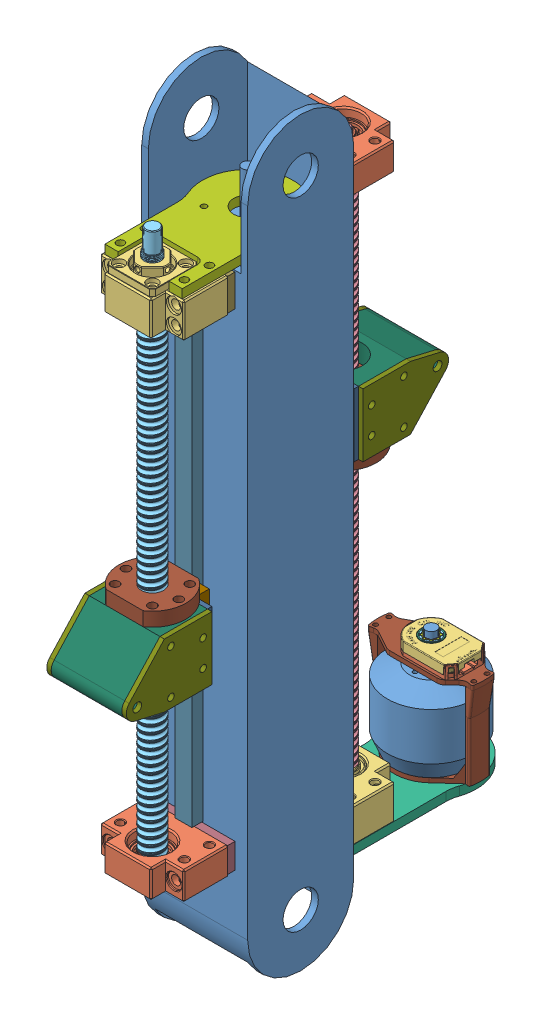
SolidWorks assembly Shoulder, configuration Default. Lengths in mm.
Overall size (98.94 533.4 280.38).
61 component instances, 29 part files, 54 mates.
Components (placement in the parent):
- Box^Shoulder-1: Box^Shoulder [Default] at origin size (76.2 533.4 76.2) (virtual)
- BF12-1: BF12 [Default] at (0 590.6294 -38.2263) x (1 0 0) z (0 1 0) size (60 43 20)
- BK12-1: BK12 [Default] at (0 188.6294 -38.2263) x (-1 0 0) z (0 -1 0) size (60 46.94 35.34)
- SFU1605-450-1: SFU1605-450 [1605-400] at (0 147.6294 -63.2263) x (1 0 0) z (0 -1 0) size (16.38 16.22 450)
- BK12-2: BK12 [Default] at (0 563.5294 48.7687) x (-1 0 0) z (0 1 0) size (60 46.94 35.34)
- BF12-2: BF12 [Default] at (0 211.5294 48.7687) x (-1 0 0) z (0 1 0) size (60 43 20)
- SFU1605-400-3: SFU1605-400 [1605-400] at (0 604.5294 73.7687) x (-1 0 0) z (0 1 0) size (16.52 16.22 400)
- J3Plate^Shoulder-1: J3Plate^Shoulder [Default] at origin size (65 6.35 120.35) (virtual)
- J2Plate^Shoulder-1: J2Plate^Shoulder [Default] at origin size (65 6.35 107.35) (virtual)
- J3MGN12R-1: J3MGN12R [Default] at origin size (12 379.5 8)
- J3MGN12C-1: J3MGN12C [Default] at (0 433.1293 -40.8288) x (1 0 0) z (0 1 0) size (27 10 45.5)
- CarriagePlate^Shoulder-1: CarriagePlate^Shoulder [Default] at (0 67.1524 5.2712) size (50.8 45.5 3.17) (virtual)
- nut-1: nut [Default] at (0 410.3793 -63.2263) x (-1 0 0) z (0 -1 0) size (48 40 42)
- BKSpacer^Shoulder-1: BKSpacer^Shoulder [Default] at origin size (58 23 5.4) (virtual)
- BKSpacer^Shoulder-2: BKSpacer^Shoulder [Default] at (0 374.9 81.5975) size (58 23 5.4) (virtual)
- BFSpacer^Shoulder-1: BFSpacer^Shoulder [Default] at origin size (58 18 5.4) (virtual)
- BFSpacer^Shoulder-2: BFSpacer^Shoulder [Default] at (0 -379.1 81.5975) size (58 18 5.4) (virtual)
- J2MGN12R^Shoulder-1: J2MGN12R^Shoulder [Default] at origin size (12 329.5 8) (virtual)
- Adapter^Shoulder-2: Adapter^Shoulder [Default] at (0 76.5186 5.2712) size (57.15 45.79 61.61) (virtual)
  - Body^Adapter_Shoulder-1: Body^Adapter_Shoulder [Default] at (38.1 26.927 0) x (0 0 -1) z (1 0 0) size (61.61 45.5 50.8) (virtual)
  - SidePlate^Adapter_Shoulder-1: SidePlate^Adapter_Shoulder [Default] at origin size (3.18 45.5 61.61) (virtual)
  - SidePlate^Adapter_Shoulder-2: SidePlate^Adapter_Shoulder [Default] at (53.975 0 0) size (3.18 45.5 61.61) (virtual)
  - 94459A340_BRASS HEAT-SET INSERT FOR PLASTIC-1: 94459A340_BRASS HEAT-SET INSERT FOR PLASTIC [94459A340] at (-18.415 340.7357 -83.735) x (0 -1 0) z (0 0 -1) size (7.22 6.55 7.22)
  - 94459A220_BRASS HEAT-SET INSERT FOR PLASTIC-1: 94459A220_BRASS HEAT-SET INSERT FOR PLASTIC [94459A220] at (13.435 346.5607 -81.9325) x (-0.837169 0 -0.546944) z (-0.546944 0 0.837169) size (8.76 13.2 8.76)
- J3MGN12C-2: J3MGN12C [Default] at (0 348.7149 51.3712) x (-1 0 0) z (0 1 0) size (27 10 45.5)
- nut-2: nut [Default] at (0 371.4649 73.7687) x (1 0 0) z (0 1 0) size (48 40 42)
- Adapter^Shoulder-3: Adapter^Shoulder [Default] at (0 705.3256 5.2712) x (1 0 0) z (0 0 -1) size (57.15 45.79 61.61) (virtual)
  - Body^Adapter_Shoulder-1: Body^Adapter_Shoulder [Default] at (38.1 26.927 0) x (0 0 -1) z (1 0 0) size (61.61 45.5 50.8) (virtual)
  - SidePlate^Adapter_Shoulder-1: SidePlate^Adapter_Shoulder [Default] at origin size (3.18 45.5 61.61) (virtual)
  - SidePlate^Adapter_Shoulder-2: SidePlate^Adapter_Shoulder [Default] at (53.975 0 0) size (3.18 45.5 61.61) (virtual)
  - 94459A340_BRASS HEAT-SET INSERT FOR PLASTIC-1: 94459A340_BRASS HEAT-SET INSERT FOR PLASTIC [94459A340] at (-18.415 340.7357 -83.735) x (0 -1 0) z (0 0 -1) size (7.22 6.55 7.22)
  - 94459A220_BRASS HEAT-SET INSERT FOR PLASTIC-1: 94459A220_BRASS HEAT-SET INSERT FOR PLASTIC [94459A220] at (13.435 346.5607 -81.9325) x (-0.837169 0 -0.546944) z (-0.546944 0 0.837169) size (8.76 13.2 8.76)
- CarriagePlate^Shoulder-2: CarriagePlate^Shoulder [Default] at (0 -17.262 5.2712) x (-1 0 0) z (0 0 -1) size (50.8 45.5 3.17) (virtual)
- MotorEncoded-1: MotorEncoded [Default] at (0 179.3044 -126.7263) x (0 0 -1) z (1 0 0) size (63 110 76.93)
  - BetterKEDA-1: BetterKEDA [Default] at origin size (63 110 63)
  - CUI_DEVICES_AMT102-0048-N2000-S-1: CUI_DEVICES_AMT102-0048-N2000-S [Default] at (0 65.12 0) x (1 0 0) z (0 1 0) size (36.33 46.21 9.2)
    - CUI_DEVICES_AMT102-0048-N2000-S.step-1: CUI_DEVICES_AMT102-0048-N2000-S.step [Default] at origin size (36.33 46.21 9.2)
      - AMT-102-Base-REV-K.step-1: AMT-102-Base-REV-K.step [Default] x (-1 0 0) z (0 0 -1) size (28.78 43.39 9.06)
      - AMT-102-Top-Cover-REV-H.step-1: AMT-102-Top-Cover-REV-H.step [Default] at (0 0 5.23) x (-1 0 0) z (0 0 -1) size (28.6 43.26 6.55)
      - AMT-Sleeve-REV-D_ 2 mm.step-1: AMT-Sleeve-REV-D_ 2 mm.step [Default] at (0 0 -2.42) x (0.999996 0.002864 0) z (0 0 1) size (10.79 10.79 7.8)
      - AMT-Hub-Top-REV-D1.step-1: AMT-Hub-Top-REV-D1.step [Default] at (0 0 2.13) x (0.999996 0.002864 0) z (0 0 1) size (14 14 5.67)
      - AMT-Hub-Bottom-REV-B.step-1: AMT-Hub-Bottom-REV-B.step [Default] at (0 0 2.43) x (0.999998 -0.001942 0) z (0 0 1) size (17.3 17.3 3.2)
      - AMT10X-Shaft-Adaptor-REV-E.step-1: AMT10X-Shaft-Adaptor-REV-E.step [Default] at (0 0 0.03) x (0.999996 0.002864 0) z (0 0 1) size (11.8 11.8 7.8)
      - Receiver-board.step-1: Receiver-board.step [Default] at (72.2834 -20.351 3.03) x (-1 0 0) z (0 0 -1) size (26.5 26.62 0.41)
      - Rotor-board-REV F.step-1: Rotor-board-REV F.step [Default] at (0 0 2.13) x (0.807874 -0.589355 0) z (0 0 1) size (26 26 0.3)
      - Transmitter-board AMT10_AMT-102.step-1: Transmitter-board AMT10_AMT-102.step [Default] at (19.1596 -17.1102 1.22) x (-1 0 0) z (0 0 -1) size (26.63 38.43 4.41)
  - Body^MotorEncoded-1: Body^MotorEncoded [Default] at origin size (53 64.53 76.93) (virtual)
- MotorEncoded-2: MotorEncoded [Default] at (0 572.8544 5.2712) x (-0.707107 0 -0.707107) z (-0.707107 0 0.707107) size (63 110 76.93)
  - BetterKEDA-1: BetterKEDA [Default] at origin size (63 110 63)
  - CUI_DEVICES_AMT102-0048-N2000-S-1: CUI_DEVICES_AMT102-0048-N2000-S [Default] at (0 65.12 0) x (1 0 0) z (0 1 0) size (36.33 46.21 9.2)
    - CUI_DEVICES_AMT102-0048-N2000-S.step-1: CUI_DEVICES_AMT102-0048-N2000-S.step [Default] at origin size (36.33 46.21 9.2)
      - AMT-102-Base-REV-K.step-1: AMT-102-Base-REV-K.step [Default] x (-1 0 0) z (0 0 -1) size (28.78 43.39 9.06)
      - AMT-102-Top-Cover-REV-H.step-1: AMT-102-Top-Cover-REV-H.step [Default] at (0 0 5.23) x (-1 0 0) z (0 0 -1) size (28.6 43.26 6.55)
      - AMT-Sleeve-REV-D_ 2 mm.step-1: AMT-Sleeve-REV-D_ 2 mm.step [Default] at (0 0 -2.42) x (0.999996 0.002864 0) z (0 0 1) size (10.79 10.79 7.8)
      - AMT-Hub-Top-REV-D1.step-1: AMT-Hub-Top-REV-D1.step [Default] at (0 0 2.13) x (0.999996 0.002864 0) z (0 0 1) size (14 14 5.67)
      - AMT-Hub-Bottom-REV-B.step-1: AMT-Hub-Bottom-REV-B.step [Default] at (0 0 2.43) x (0.999998 -0.001942 0) z (0 0 1) size (17.3 17.3 3.2)
      - AMT10X-Shaft-Adaptor-REV-E.step-1: AMT10X-Shaft-Adaptor-REV-E.step [Default] at (0 0 0.03) x (0.999996 0.002864 0) z (0 0 1) size (11.8 11.8 7.8)
      - Receiver-board.step-1: Receiver-board.step [Default] at (72.2834 -20.351 3.03) x (-1 0 0) z (0 0 -1) size (26.5 26.62 0.41)
      - Rotor-board-REV F.step-1: Rotor-board-REV F.step [Default] at (0 0 2.13) x (0.807874 -0.589355 0) z (0 0 1) size (26 26 0.3)
      - Transmitter-board AMT10_AMT-102.step-1: Transmitter-board AMT10_AMT-102.step [Default] at (19.1596 -17.1102 1.22) x (-1 0 0) z (0 0 -1) size (26.63 38.43 4.41)
  - Body^MotorEncoded-1: Body^MotorEncoded [Default] at origin size (53 64.53 76.93) (virtual)
Mates (geometry in assembly coordinates):
- Parallel1: parallel anti-aligned: plane of Box^Shoulder-1 through (-33.3375 163.4294 -32.8288) normal (0 0 -1); plane of BF12-1 through (29 581.6294 -38.2263) normal (0 0 1)
- Width1: width anti-aligned: plane of BF12-1 through (30 581.6294 -69.7263) normal (1 0 0); plane of BF12-1 through (-30 581.6294 -39.2263) normal (-1 0 0); plane of Box^Shoulder-1 through (38.1 620.6294 5.2712) normal (1 0 0); plane of Box^Shoulder-1 through (-38.1 163.4294 5.2712) normal (-1 0 0)
- Distance6: distance anti-aligned: plane of Box^Shoulder-1 through (-33.3375 163.4294 -32.8288) normal (0 0 -1); plane of BK12-1 through (-29 200.1294 -38.2263) normal (0 0 1)
- Width2: width aligned: plane of BK12-1 through (30 200.1294 -39.2263) normal (1 0 0); plane of BK12-1 through (-30 200.1294 -69.7263) normal (-1 0 0); plane of Box^Shoulder-1 through (-38.1 163.4294 5.2712) normal (-1 0 0); plane of Box^Shoulder-1 through (38.1 620.6294 5.2712) normal (1 0 0)
- Parallel3: parallel aligned: plane of BK12-1 through (29 201.1294 -39.2263) normal (0 1 0)
- Coincident11: coincident: line of SFU1605-450-1 through (0 162.3794 -63.2263) axis (0 -1 0)
- Concentric6: concentric anti-aligned: cylinder of BK12-1 through (0 196.6294 -63.2263) axis (0 1 0) radius 6; cylinder of SFU1605-450-1 through (0 162.6294 -63.2263) axis (0 -1 0) radius 5
- Coincident12: coincident anti-aligned: plane of BK12-1 through (7.2358 201.6294 -55.9905) normal (0 1 0); plane of SFU1605-450-1 through (0 201.6294 -63.2263) normal (0 -1 0)
- Coincident13: coincident anti-aligned: plane of BF12-1 through (-6.5021 586.6294 -56.7242) normal (0 -1 0); plane of SFU1605-450-1 through (0 586.6294 -63.2263) normal (0 1 0)
- Distance3: distance = 12.7 mm: plane of BK12-1 through (29 176.1294 -39.2263) normal (0 -1 0); line of Box^Shoulder-1 through (38.1 163.4294 -32.8288) axis (-1 0 0)
- Coincident27: coincident: line of SFU1605-400-3 through (0 589.7794 73.7687) axis (0 1 0)
- Concentric18: concentric anti-aligned: cylinder of BK12-2 through (0 563.5294 73.7687) axis (0 -1 0) radius 6; cylinder of SFU1605-400-3 through (0 589.5294 73.7687) axis (0 1 0) radius 5
- Distance8: distance anti-aligned: plane of Box^Shoulder-1 through (-33.3375 163.4294 43.3712) normal (0 0 1); plane of BK12-2 through (-29 552.0294 48.7687) normal (0 0 -1)
- Coincident29: coincident anti-aligned: plane of BK12-2 through (7.2358 550.5294 66.5329) normal (0 -1 0); plane of SFU1605-400-3 through (0 550.5294 73.7687) normal (0 1 0)
- Coincident30: coincident anti-aligned: plane of BF12-2 through (-6.5021 215.5294 67.2666) normal (0 1 0); plane of SFU1605-400-3 through (0 215.5294 73.7687) normal (0 -1 0)
- Concentric19: concentric anti-aligned: cylinder of BF12-2 through (0 208.3294 73.7687) axis (0 1 0) radius 5; cylinder of SFU1605-400-3 through (0 215.5294 73.7687) axis (0 -1 0) radius 5
- Distance5: distance = 38.1 mm: line of Box^Shoulder-1 through (38.1 163.4294 43.3712) axis (-1 0 0); plane of BF12-2 through (29 201.5294 49.7687) normal (0 -1 0)
- Coincident35: coincident anti-aligned: plane of J3MGN12R-1 through (0 0 -40.8288) normal (0 0 -1); plane of J3MGN12C-1 through (-6 455.8793 -40.8288) normal (0 0 1)
- Width3: width anti-aligned: plane of J3MGN12C-1 through (13.5 455.8793 -35.8288) normal (1 0 0); plane of J3MGN12R-1 through (-13.5 455.8793 -35.8288) normal (-1 0 0); plane of J3MGN12C-1 through (-6 580.6294 -40.8288) normal (-1 0 0); plane of J3MGN12R-1 through (6 580.6294 -40.8288) normal (1 0 0)
- Coincident36: coincident anti-aligned: plane of J3MGN12C-1 through (13.5 455.8793 -45.8288) normal (0 0 -1); plane of CarriagePlate^Shoulder-1 through (0 67.1524 -45.8288) normal (0 0 1)
- Concentric22: concentric anti-aligned: cylinder of J3MGN12C-1 through (10 443.1293 -41.8288) axis (0 0 -1) radius 1.5; cylinder of CarriagePlate^Shoulder-1 through (10 443.1293 -49.0038) axis (0 0 1) radius 1.5
- Concentric23: concentric anti-aligned: cylinder of J3MGN12C-1 through (-10 423.1293 -41.8288) axis (0 0 -1) radius 1.5; cylinder of CarriagePlate^Shoulder-1 through (-10 423.1293 -49.0038) axis (0 0 1) radius 1.5
- Concentric24: concentric aligned: cylinder of SFU1605-450-1 through (0 586.6294 -63.2263) axis (0 1 0) radius 5; cylinder of nut-1 through (0 400.3793 -63.2263) axis (0 1 0) radius 8
- Concentric25: concentric aligned: cylinder of BF12-1 through (0 587.4294 -63.2263) axis (0 1 0) radius 5; cylinder of SFU1605-450-1 through (0 586.6294 -63.2263) axis (0 1 0) radius 5
- Coincident37: coincident anti-aligned: plane of CarriagePlate^Shoulder-1 through (-25.4 410.3793 -49.0038) normal (0 -1 0); plane of nut-1 through (0 410.3793 -63.2263) normal (0 1 0)
- Parallel4: parallel anti-aligned: plane of Box^Shoulder-1 through (-33.3375 163.4294 43.3712) normal (0 0 1); plane of BF12-2 through (-29 202.5294 48.7687) normal (0 0 -1)
- Concentric27: concentric anti-aligned: cylinder of BK12-2 through (-23 557.0294 48.7687) axis (0 0 1) radius 3.3; cylinder of BKSpacer^Shoulder-2 through (-23 557.0294 111.1626) axis (0 0 -1) radius 3.3
- Concentric28: concentric anti-aligned: cylinder of BK12-2 through (23 557.0294 48.7687) axis (0 0 1) radius 3.3; cylinder of BKSpacer^Shoulder-2 through (23 557.0294 111.1626) axis (0 0 -1) radius 3.3
- Coincident42: coincident anti-aligned: plane of Box^Shoulder-1 through (-33.3375 163.4294 43.3712) normal (0 0 1); plane of BKSpacer^Shoulder-2 through (0 374.9 43.3712) normal (0 0 -1)
- Concentric29: concentric anti-aligned: cylinder of BF12-2 through (23 211.5294 48.7687) axis (0 0 1) radius 3.3; cylinder of BFSpacer^Shoulder-2 through (23 211.5294 109.4976) axis (0 0 -1) radius 3.3
- Concentric30: concentric anti-aligned: cylinder of BF12-2 through (-23 211.5294 48.7687) axis (0 0 1) radius 3.3; cylinder of BFSpacer^Shoulder-2 through (-23 211.5294 109.4976) axis (0 0 -1) radius 3.3
- Coincident43: coincident anti-aligned: plane of Box^Shoulder-1 through (-33.3375 163.4294 43.3712) normal (0 0 1); plane of BFSpacer^Shoulder-2 through (0 -379.1 43.3712) normal (0 0 -1)
- Concentric32: concentric anti-aligned: cylinder of nut-1 through (0 442.3793 -63.2263) axis (0 -1 0) radius 14; cylinder of Adapter^Shoulder-2/Body^Adapter_Shoulder-1 through (0 349.1272 -63.2263) axis (0 1 0) radius 14
- Parallel6: parallel anti-aligned: plane of CarriagePlate^Shoulder-1 through (0 67.1524 -49.0038) normal (0 0 -1); plane of Adapter^Shoulder-2/Body^Adapter_Shoulder-1 through (38.1 349.1272 -49.0038) normal (0 0 1)
- Coincident47: coincident anti-aligned: plane of nut-1 through (0 410.3793 -63.2263) normal (0 1 0); plane of Adapter^Shoulder-2/Body^Adapter_Shoulder-1 through (-25.4 410.3793 -49.0038) normal (0 -1 0)
- Coincident48: coincident anti-aligned: plane of nut-1 through (0 410.3793 -63.2263) normal (0 1 0); plane of Adapter^Shoulder-2/Body^Adapter_Shoulder-1 through (-25.4 410.3793 -49.0038) normal (0 -1 0)
- Coincident49: coincident anti-aligned: plane of nut-1 through (0 410.3793 -63.2263) normal (0 1 0); plane of Adapter^Shoulder-2/Body^Adapter_Shoulder-1 through (-25.4 410.3793 -49.0038) normal (0 -1 0)
- Coincident51: coincident anti-aligned: plane of J2MGN12R^Shoulder-1 through (0 0 51.3712) normal (0 0 1); plane of J3MGN12C-2 through (6 371.4649 51.3712) normal (0 0 -1)
- Width6: width anti-aligned: plane of J3MGN12C-2 through (-13.5 371.4649 46.3712) normal (-1 0 0); plane of J2MGN12R^Shoulder-1 through (13.5 371.4649 46.3712) normal (1 0 0); plane of J3MGN12C-2 through (6 551.0294 51.3712) normal (1 0 0); plane of J2MGN12R^Shoulder-1 through (-6 551.0294 51.3712) normal (-1 0 0)
- Concentric34: concentric anti-aligned: cylinder of SFU1605-400-3 through (0 589.5294 73.7687) axis (0 1 0) radius 5; cylinder of nut-2 through (0 381.4649 73.7687) axis (0 -1 0) radius 8
- Coincident52: coincident anti-aligned: plane of J3MGN12C-2 through (0 371.4649 51.3712) normal (0 1 0); plane of nut-2 through (0 371.4649 73.7687) normal (0 -1 0)
- Concentric35: concentric anti-aligned: cylinder of nut-2 through (0 339.4649 73.7687) axis (0 1 0) radius 14; cylinder of Adapter^Shoulder-3/Body^Adapter_Shoulder-1 through (0 432.717 73.7687) axis (0 -1 0) radius 14
- Parallel7: parallel anti-aligned: plane of J3MGN12C-2 through (-13.5 371.4649 56.3712) normal (0 0 1); plane of Adapter^Shoulder-3/Body^Adapter_Shoulder-1 through (38.1 432.717 59.5462) normal (0 0 -1)
- Coincident54: coincident anti-aligned: plane of nut-2 through (0 371.4649 73.7687) normal (0 -1 0); plane of Adapter^Shoulder-3/Body^Adapter_Shoulder-1 through (-25.4 371.4649 59.5462) normal (0 1 0)
- Concentric36: concentric anti-aligned: cylinder of J3MGN12C-2 through (10 358.7149 52.3712) axis (0 0 1) radius 1.5; cylinder of CarriagePlate^Shoulder-2 through (10 358.7149 59.5462) axis (0 0 -1) radius 1.5
- Concentric37: concentric anti-aligned: cylinder of J3MGN12C-2 through (-10 338.7149 52.3712) axis (0 0 1) radius 1.5; cylinder of CarriagePlate^Shoulder-2 through (-10 338.7149 59.5462) axis (0 0 -1) radius 1.5
- Coincident55: coincident anti-aligned: plane of J3MGN12C-2 through (-13.5 371.4649 56.3712) normal (0 0 1); plane of CarriagePlate^Shoulder-2 through (0 -17.262 56.3712) normal (0 0 -1)
- Parallel8: parallel aligned: plane of BF12-2 through (29 221.5294 49.7687) normal (0 1 0)
- Concentric38: concentric aligned: cylinder of J3Plate^Shoulder-1 through (0 169.7794 -126.7263) axis (0 1 0) radius 8; cylinder of MotorEncoded-1/BetterKEDA-1 through (0 144.3044 -126.7263) axis (0 1 0) radius 4
- Concentric39: concentric aligned: cylinder of J3Plate^Shoulder-1 through (0 169.7794 -104.5263) axis (0 1 0) radius 2; cylinder of MotorEncoded-1/Body^MotorEncoded-1 through (0 176.1294 -104.5263) axis (0 1 0) radius 2
- Coincident56: coincident anti-aligned: plane of J3Plate^Shoulder-1 through (54.75 176.1294 -107.8889) normal (0 1 0); plane of MotorEncoded-1/Body^MotorEncoded-1 through (0 176.1294 -126.7263) normal (0 -1 0)
- Concentric40: concentric aligned: cylinder of J2Plate^Shoulder-1 through (0 582.3794 5.2712) axis (0 -1 0) radius 10; cylinder of MotorEncoded-2/BetterKEDA-1 through (0 607.8544 5.2712) axis (0 -1 0) radius 4
- Concentric41: concentric aligned: cylinder of J2Plate^Shoulder-1 through (-15.6978 582.3794 20.9689) axis (0 -1 0) radius 2; cylinder of MotorEncoded-2/Body^MotorEncoded-1 through (-15.6978 576.0294 20.9689) axis (0 -1 0) radius 2
- Coincident57: coincident anti-aligned: plane of J2Plate^Shoulder-1 through (0 576.0294 0) normal (0 -1 0); plane of MotorEncoded-2/Body^MotorEncoded-1 through (0 576.0294 5.2712) normal (0 1 0)
